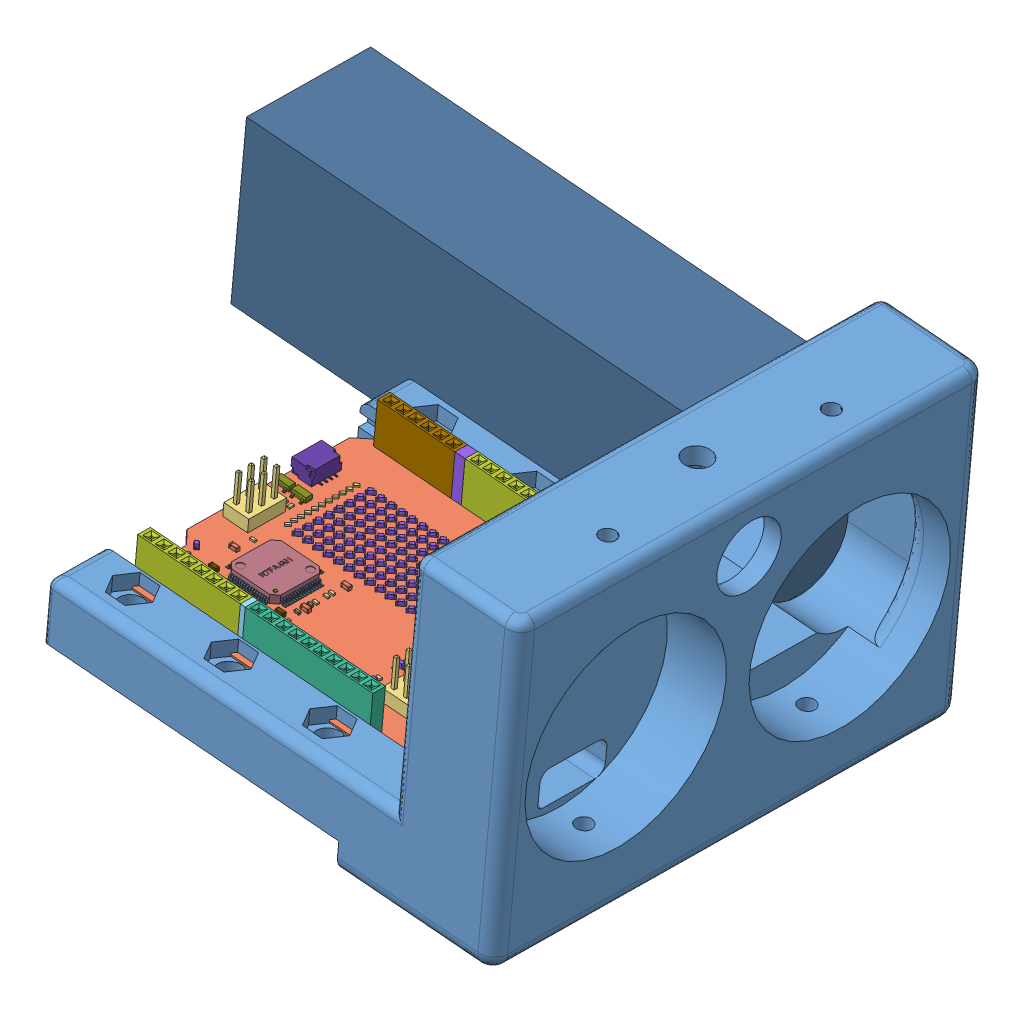
SolidWorks assembly SensorboxController1, configuration Standard. Lengths in mm. (continued)
Components (placement in the parent): (continued)
- PCB(ABX00087).step-1: PCB(ABX00087).step [Standard] at (42.9255 -81.7651 134.9822) x (-0.996616 0.082156 -0.002776) z (0.08218 0.996566 -0.010101) size (70.54 53.34 14.5) (continued)
  - U4.step-1: U4.step [Standard] at origin size (4 2 0.55) (continued)
    - IC_Texas_Instruments_TXB0108DQSR_eec.step-1: IC_Texas_Instruments_TXB0108DQSR_eec.step [Standard] at (13.565 34.6878 0.3) x (1 0 0) z (0 0 1) size (4 2 0.55) (continued)
      - Part16_MIR.step-2: Part16_MIR.step [Standard] at (3.331 -0.6643 -0.3) x (1 0 0) z (0 0 -1) size (0.2 0.55 0.1)
      - Part16_MIR1.step-1: Part16_MIR1.step [Standard] at (4.131 -0.6643 -0.3) x (1 0 0) z (0 0 -1) size (0.2 0.55 0.1)
      - Part16_MIR1.step-2: Part16_MIR1.step [Standard] at (4.531 -0.6643 -0.3) x (1 0 0) z (0 0 -1) size (0.2 0.55 0.1)
      - Part16_MIR1.step-3: Part16_MIR1.step [Standard] at (4.931 -0.6643 -0.3) x (1 0 0) z (0 0 -1) size (0.2 0.55 0.1)
      - Part16_MIR1.step-4: Part16_MIR1.step [Standard] at (5.331 -0.6643 -0.3) x (1 0 0) z (0 0 -1) size (0.2 0.55 0.1)
      - Part16_MIR1.step-5: Part16_MIR1.step [Standard] at (5.731 -0.6643 -0.3) x (1 0 0) z (0 0 -1) size (0.2 0.55 0.1)
      - Part16_MIR1.step-6: Part16_MIR1.step [Standard] at (6.131 -0.6643 -0.3) x (1 0 0) z (0 0 -1) size (0.2 0.55 0.1)
      - Part16_MIR1.step-7: Part16_MIR1.step [Standard] at (6.531 -0.6643 -0.3) x (1 0 0) z (0 0 -1) size (0.2 0.55 0.1)
      - Part16_MIR1.step-8: Part16_MIR1.step [Standard] at (6.931 -0.6643 -0.3) x (1 0 0) z (0 0 -1) size (0.2 0.55 0.1)
      - Part16 - Copy.step-1: Part16 - Copy.step [Standard] at (3.331 -2.0643 -0.3) size (0.2 0.65 0.1)
  - C24.step-1: C24.step [Standard] at origin size (0.5 1 0.5)
    - CAP-0402.step-1: CAP-0402.step [Standard] at (18.146 36.576 0) x (0 -1 0) z (0 0 1) size (1 0.5 0.5)
  - C25.step-1: C25.step [Standard] at origin size (0.5 1 0.5)
    - CAP-0402.step-1: CAP-0402.step [Standard] at (19.246 36.576 0) x (0 -1 0) z (0 0 1) size (1 0.5 0.5)
  - C26.step-1: C26.step [Standard] at origin size (0.5 1 0.5)
    - CAP-0402.step-1: CAP-0402.step [Standard] at (15.796 33.276 0) x (0 1 0) z (0 0 1) size (1 0.5 0.5)
  - U3.step-1: U3.step [Standard] at origin size (4 3 1)
    - 6430905744.step-1: 6430905744.step [Standard] at (26.825 22.1 0) x (0 1 0) z (0 0 1) size (3 4 1)
      - Body-3.step-1: Body-3.step [Standard] at (-1.5 -2 0) size (3 4 1)
        - Open CASCADE STEP translator 6.8 36.2.1.step-1: Open CASCADE STEP translator 6.8 36.2.1.step [Standard] at origin size (3 4 1)
      - Pin_Shape.step-1: Pin_Shape.step [Standard] at (-1.5 -1.3675 0) size (0.4 0.23 0.2)
        - Open CASCADE STEP translator 6.8 36.4.1.step-1: Open CASCADE STEP translator 6.8 36.4.1.step [Standard] at origin size (0.4 0.23 0.2)
      - Pin_Shape.step-2: Pin_Shape.step [Standard] at (1.5 1.3675 0) x (-1 0 0) z (0 0 1) size (0.4 0.23 0.2)
        - Open CASCADE STEP translator 6.8 36.4.1.step-1: Open CASCADE STEP translator 6.8 36.4.1.step [Standard] at origin size (0.4 0.23 0.2)
      - Pin_Shape.step-3: Pin_Shape.step [Standard] at (-1.5 -0.8675 0) size (0.4 0.23 0.2)
        - Open CASCADE STEP translator 6.8 36.4.1.step-1: Open CASCADE STEP translator 6.8 36.4.1.step [Standard] at origin size (0.4 0.23 0.2)
      - Pin_Shape.step-4: Pin_Shape.step [Standard] at (1.5 0.8675 0) x (-1 0 0) z (0 0 1) size (0.4 0.23 0.2)
        - Open CASCADE STEP translator 6.8 36.4.1.step-1: Open CASCADE STEP translator 6.8 36.4.1.step [Standard] at origin size (0.4 0.23 0.2)
      - Pin_Shape.step-5: Pin_Shape.step [Standard] at (-1.5 -0.3675 0) size (0.4 0.23 0.2)
        - Open CASCADE STEP translator 6.8 36.4.1.step-1: Open CASCADE STEP translator 6.8 36.4.1.step [Standard] at origin size (0.4 0.23 0.2)
      - Pin_Shape.step-6: Pin_Shape.step [Standard] at (1.5 0.3675 0) x (-1 0 0) z (0 0 1) size (0.4 0.23 0.2)
        - Open CASCADE STEP translator 6.8 36.4.1.step-1: Open CASCADE STEP translator 6.8 36.4.1.step [Standard] at origin size (0.4 0.23 0.2)
      - Pin_Shape.step-7: Pin_Shape.step [Standard] at (-1.5 0.1325 0) size (0.4 0.23 0.2)
        - Open CASCADE STEP translator 6.8 36.4.1.step-1: Open CASCADE STEP translator 6.8 36.4.1.step [Standard] at origin size (0.4 0.23 0.2)
      - Pin_Shape.step-8: Pin_Shape.step [Standard] at (1.5 -0.1325 0) x (-1 0 0) z (0 0 1) size (0.4 0.23 0.2)
        - Open CASCADE STEP translator 6.8 36.4.1.step-1: Open CASCADE STEP translator 6.8 36.4.1.step [Standard] at origin size (0.4 0.23 0.2)
      - Pin_Shape.step-9: Pin_Shape.step [Standard] at (-1.5 0.6325 0) size (0.4 0.23 0.2)
        - Open CASCADE STEP translator 6.8 36.4.1.step-1: Open CASCADE STEP translator 6.8 36.4.1.step [Standard] at origin size (0.4 0.23 0.2)
      - Pin_Shape.step-10: Pin_Shape.step [Standard] at (1.5 -0.6325 0) x (-1 0 0) z (0 0 1) size (0.4 0.23 0.2)
        - Open CASCADE STEP translator 6.8 36.4.1.step-1: Open CASCADE STEP translator 6.8 36.4.1.step [Standard] at origin size (0.4 0.23 0.2)
      - Pin_Shape.step-11: Pin_Shape.step [Standard] at (-1.5 1.1325 0) size (0.4 0.23 0.2)
        - Open CASCADE STEP translator 6.8 36.4.1.step-1: Open CASCADE STEP translator 6.8 36.4.1.step [Standard] at origin size (0.4 0.23 0.2)
      - Pin_Shape.step-12: Pin_Shape.step [Standard] at (1.5 -1.1325 0) x (-1 0 0) z (0 0 1) size (0.4 0.23 0.2)
        - Open CASCADE STEP translator 6.8 36.4.1.step-1: Open CASCADE STEP translator 6.8 36.4.1.step [Standard] at origin size (0.4 0.23 0.2)
      - Open CASCADE STEP translator 6.8 36.1.step-1: Open CASCADE STEP translator 6.8 36.1.step [Standard] at (-1.5 -2 0) size (0.38 0.38 0)
      - Thermal_Shape.step-1: Thermal_Shape.step [Standard] at (-0.8375 -1.6375 -0.001) size (1.68 3.28 0)
  - U1.step-1: U1.step [Standard] at origin size (12.2 12.2 1.68)
    - RA4M1 v4.step-1: RA4M1 v4.step [Standard] at (40.7498 25.853 0) size (12.2 12.2 1.67)
      - Designator1.step-1: Designator1.step [Standard] at origin size (12.2 12.2 1.67)
        - 6422462560.step-1: 6422462560.step [Standard] at (12 10 0) size (12.2 12.2 1.65)
          - Body-4.step-1: Body-4.step [Standard] at (-5 -5 0) size (10 10 1.65)
            - Open CASCADE STEP translator 6.8 23.1.1.step-1: Open CASCADE STEP translator 6.8 23.1.1.step [Standard] at origin size (10 10 1.65)
          - Leader-2.step-1: Leader-2.step [Standard] at (-5 -3.75 0) x (-1 0 0) z (0 0 1) size (1.1 0.27 0.88)
          - Leader-2.step-2: Leader-2.step [Standard] at (-3.75 5 0) x (0 1 0) z (0 0 1) size (1.1 0.27 0.88)
          - Leader-2.step-3: Leader-2.step [Standard] at (5 -3.75 0) size (1.1 0.27 0.88)
          - Leader-2.step-4: Leader-2.step [Standard] at (-3.75 -5 0) x (0 -1 0) z (0 0 1) size (1.1 0.27 0.88)
          - Leader-2.step-5: Leader-2.step [Standard] at (-5 -3.25 0) x (-1 0 0) z (0 0 1) size (1.1 0.27 0.88)
          - Leader-2.step-6: Leader-2.step [Standard] at (-3.25 5 0) x (0 1 0) z (0 0 1) size (1.1 0.27 0.88)
          - Leader-2.step-7: Leader-2.step [Standard] at (5 -3.25 0) size (1.1 0.27 0.88)
          - Leader-2.step-8: Leader-2.step [Standard] at (-3.25 -5 0) x (0 -1 0) z (0 0 1) size (1.1 0.27 0.88)
          - Leader-2.step-9: Leader-2.step [Standard] at (-5 -2.75 0) x (-1 0 0) z (0 0 1) size (1.1 0.27 0.88)
          - Leader-2.step-10: Leader-2.step [Standard] at (-2.75 5 0) x (0 1 0) z (0 0 1) size (1.1 0.27 0.88)
          - Leader-2.step-11: Leader-2.step [Standard] at (5 -2.75 0) size (1.1 0.27 0.88)
          - Leader-2.step-12: Leader-2.step [Standard] at (-2.75 -5 0) x (0 -1 0) z (0 0 1) size (1.1 0.27 0.88)
          - Leader-2.step-13: Leader-2.step [Standard] at (-5 -2.25 0) x (-1 0 0) z (0 0 1) size (1.1 0.27 0.88)
          - Leader-2.step-14: Leader-2.step [Standard] at (-2.25 5 0) x (0 1 0) z (0 0 1) size (1.1 0.27 0.88)
          - Leader-2.step-15: Leader-2.step [Standard] at (5 -2.25 0) size (1.1 0.27 0.88)
          - Leader-2.step-16: Leader-2.step [Standard] at (-2.25 -5 0) x (0 -1 0) z (0 0 1) size (1.1 0.27 0.88)
          - Leader-2.step-17: Leader-2.step [Standard] at (-5 -1.75 0) x (-1 0 0) z (0 0 1) size (1.1 0.27 0.88)
          - Leader-2.step-18: Leader-2.step [Standard] at (-1.75 5 0) x (0 1 0) z (0 0 1) size (1.1 0.27 0.88)
          - Leader-2.step-19: Leader-2.step [Standard] at (5 -1.75 0) size (1.1 0.27 0.88)
          - Leader-2.step-20: Leader-2.step [Standard] at (-1.75 -5 0) x (0 -1 0) z (0 0 1) size (1.1 0.27 0.88)
          - Leader-2.step-21: Leader-2.step [Standard] at (-5 -1.25 0) x (-1 0 0) z (0 0 1) size (1.1 0.27 0.88)
          - Leader-2.step-22: Leader-2.step [Standard] at (-1.25 5 0) x (0 1 0) z (0 0 1) size (1.1 0.27 0.88)
          - Leader-2.step-23: Leader-2.step [Standard] at (5 -1.25 0) size (1.1 0.27 0.88)
          - Leader-2.step-24: Leader-2.step [Standard] at (-1.25 -5 0) x (0 -1 0) z (0 0 1) size (1.1 0.27 0.88)
          - Leader-2.step-25: Leader-2.step [Standard] at (-5 -0.75 0) x (-1 0 0) z (0 0 1) size (1.1 0.27 0.88)
          - Leader-2.step-26: Leader-2.step [Standard] at (-0.75 5 0) x (0 1 0) z (0 0 1) size (1.1 0.27 0.88)
          - Leader-2.step-27: Leader-2.step [Standard] at (5 -0.75 0) size (1.1 0.27 0.88)
          - Leader-2.step-28: Leader-2.step [Standard] at (-0.75 -5 0) x (0 -1 0) z (0 0 1) size (1.1 0.27 0.88)
          - Leader-2.step-29: Leader-2.step [Standard] at (-5 -0.25 0) x (-1 0 0) z (0 0 1) size (1.1 0.27 0.88)
          - Leader-2.step-30: Leader-2.step [Standard] at (-0.25 5 0) x (0 1 0) z (0 0 1) size (1.1 0.27 0.88)
          - Leader-2.step-31: Leader-2.step [Standard] at (5 -0.25 0) size (1.1 0.27 0.88)
          - Leader-2.step-32: Leader-2.step [Standard] at (-0.25 -5 0) x (0 -1 0) z (0 0 1) size (1.1 0.27 0.88)
          - Leader-2.step-33: Leader-2.step [Standard] at (-5 0.25 0) x (-1 0 0) z (0 0 1) size (1.1 0.27 0.88)
          - Leader-2.step-34: Leader-2.step [Standard] at (0.25 5 0) x (0 1 0) z (0 0 1) size (1.1 0.27 0.88)
          - Leader-2.step-35: Leader-2.step [Standard] at (5 0.25 0) size (1.1 0.27 0.88)
          - Leader-2.step-36: Leader-2.step [Standard] at (0.25 -5 0) x (0 -1 0) z (0 0 1) size (1.1 0.27 0.88)
          - Leader-2.step-37: Leader-2.step [Standard] at (-5 0.75 0) x (-1 0 0) z (0 0 1) size (1.1 0.27 0.88)
          - Leader-2.step-38: Leader-2.step [Standard] at (0.75 5 0) x (0 1 0) z (0 0 1) size (1.1 0.27 0.88)
          - Leader-2.step-39: Leader-2.step [Standard] at (5 0.75 0) size (1.1 0.27 0.88)
          - Leader-2.step-40: Leader-2.step [Standard] at (0.75 -5 0) x (0 -1 0) z (0 0 1) size (1.1 0.27 0.88)
          - Leader-2.step-41: Leader-2.step [Standard] at (-5 1.25 0) x (-1 0 0) z (0 0 1) size (1.1 0.27 0.88)
          - Leader-2.step-42: Leader-2.step [Standard] at (1.25 5 0) x (0 1 0) z (0 0 1) size (1.1 0.27 0.88)
          - Leader-2.step-43: Leader-2.step [Standard] at (5 1.25 0) size (1.1 0.27 0.88)
          - Leader-2.step-44: Leader-2.step [Standard] at (1.25 -5 0) x (0 -1 0) z (0 0 1) size (1.1 0.27 0.88)
          - Leader-2.step-45: Leader-2.step [Standard] at (-5 1.75 0) x (-1 0 0) z (0 0 1) size (1.1 0.27 0.88)
          - Leader-2.step-46: Leader-2.step [Standard] at (1.75 5 0) x (0 1 0) z (0 0 1) size (1.1 0.27 0.88)
          - Leader-2.step-47: Leader-2.step [Standard] at (5 1.75 0) size (1.1 0.27 0.88)
          - Leader-2.step-48: Leader-2.step [Standard] at (1.75 -5 0) x (0 -1 0) z (0 0 1) size (1.1 0.27 0.88)
          - Leader-2.step-49: Leader-2.step [Standard] at (-5 2.25 0) x (-1 0 0) z (0 0 1) size (1.1 0.27 0.88)
          - Leader-2.step-50: Leader-2.step [Standard] at (2.25 5 0) x (0 1 0) z (0 0 1) size (1.1 0.27 0.88)
          - Leader-2.step-51: Leader-2.step [Standard] at (5 2.25 0) size (1.1 0.27 0.88)
          - Leader-2.step-52: Leader-2.step [Standard] at (2.25 -5 0) x (0 -1 0) z (0 0 1) size (1.1 0.27 0.88)
          - Leader-2.step-53: Leader-2.step [Standard] at (-5 2.75 0) x (-1 0 0) z (0 0 1) size (1.1 0.27 0.88)
          - Leader-2.step-54: Leader-2.step [Standard] at (2.75 5 0) x (0 1 0) z (0 0 1) size (1.1 0.27 0.88)
          - Leader-2.step-55: Leader-2.step [Standard] at (5 2.75 0) size (1.1 0.27 0.88)
          - Leader-2.step-56: Leader-2.step [Standard] at (2.75 -5 0) x (0 -1 0) z (0 0 1) size (1.1 0.27 0.88)
          - Leader-2.step-57: Leader-2.step [Standard] at (-5 3.25 0) x (-1 0 0) z (0 0 1) size (1.1 0.27 0.88)
          - Leader-2.step-58: Leader-2.step [Standard] at (3.25 5 0) x (0 1 0) z (0 0 1) size (1.1 0.27 0.88)
          - Leader-2.step-59: Leader-2.step [Standard] at (5 3.25 0) size (1.1 0.27 0.88)
          - Leader-2.step-60: Leader-2.step [Standard] at (3.25 -5 0) x (0 -1 0) z (0 0 1) size (1.1 0.27 0.88)
          - Leader-2.step-61: Leader-2.step [Standard] at (-5 3.75 0) x (-1 0 0) z (0 0 1) size (1.1 0.27 0.88)
          - Leader-2.step-62: Leader-2.step [Standard] at (3.75 5 0) x (0 1 0) z (0 0 1) size (1.1 0.27 0.88)
          - Leader-2.step-63: Leader-2.step [Standard] at (5 3.75 0) size (1.1 0.27 0.88)
          - Leader-2.step-64: Leader-2.step [Standard] at (3.75 -5 0) x (0 -1 0) z (0 0 1) size (1.1 0.27 0.88)
        - 7219473552.step-1: 7219473552.step [Standard] at (8.2001 13.7999 0.25) size (0.7 0.7 1.42)
          - Extruded-3.step-1: Extruded-3.step [Standard] at origin size (0.7 0.7 1.42)
    - 6360838992.step-1: 6360838992.step [Standard] at (48.9498 39.6529 0.25) size (0.7 0.71 1.43)
      - Extruded-4.step-1: Extruded-4.step [Standard] at origin size (0.7 0.71 1.43)
  - R23.step-1: R23.step [Standard] at origin size (1 0.5 0.34)
    - RES-0402.step-1: RES-0402.step [Standard] at (26.416 35.433 0) size (1 0.5 0.34)
  - R40.step-1: R40.step [Standard] at origin size (0.5 1 0.34)
    - RES-0402.step-1: RES-0402.step [Standard] at (25.125 25.3 0) x (0 -1 0) z (0 0 1) size (1 0.5 0.34)
  - R38.step-1: R38.step [Standard] at origin size (0.5 1 0.34)
    - RES-0402.step-1: RES-0402.step [Standard] at (26.225 25.3 0) x (0 -1 0) z (0 0 1) size (1 0.5 0.34)
  - R36.step-1: R36.step [Standard] at origin size (1 0.5 0.34)
    - RES-0402.step-1: RES-0402.step [Standard] at (27.95 27.235 0) x (-1 0 0) z (0 0 1) size (1 0.5 0.34)
  - R44.step-1: R44.step [Standard] at origin size (0.5 1 0.34)
    - RES-0402.step-1: RES-0402.step [Standard] at (22.925 23 0) x (0 1 0) z (0 0 1) size (1 0.5 0.34)
  - R43.step-1: R43.step [Standard] at origin size (0.5 1 0.34)
    - RES-0402.step-1: RES-0402.step [Standard] at (22.925 25.3 0) x (0 -1 0) z (0 0 1) size (1 0.5 0.34)
  - R7.step-1: R7.step [Standard] at origin size (1 0.5 0.34)
    - RES-0402.step-1: RES-0402.step [Standard] at (60.646 32.376 0) x (-1 0 0) z (0 0 1) size (1 0.5 0.34)
  - R1.step-1: R1.step [Standard] at origin size (0.5 1 0.34)
    - RES-0402.step-1: RES-0402.step [Standard] at (13.125 34.231 0) x (0 1 0) z (0 0 1) size (1 0.5 0.34)
  - L3.step-1: L3.step [Standard] at origin size (4.8 4.8 2)
    - 6431045296.step-1: 6431045296.step [Standard] at (29.5083 17.2482 0.05) size (4.8 4.8 2)
      - Extruded-5.step-1: Extruded-5.step [Standard] at origin size (4.8 4.8 2)
  - L2.step-1: L2.step [Standard] at origin size (1.6 0.8 0.8)
    - FER-0603.step-1: FER-0603.step [Standard] at (59.5098 41.428 0) x (1 0 0) z (0 0 1) size (1.6 0.8 0.8)
  - L1.step-1: L1.step [Standard] at origin size (1.6 0.8 0.8)
    - FER-0603.step-1: FER-0603.step [Standard] at (45.9897 41.428 0) x (1 0 0) z (0 0 1) size (1.6 0.8 0.8)
  - C16.step-1: C16.step [Standard] at origin size (2 1.25 1.25)
    - CAP-0805.step-1: CAP-0805.step [Standard] at (30.6599 23.2481 0) x (-1 0 0) z (0 0 1) size (2 1.25 1.25)
  - C11.step-1: C11.step [Standard] at origin size (0.5 1 0.5)
    - CAP-0402.step-1: CAP-0402.step [Standard] at (19.19 9.991 0) x (0 1 0) z (0 0 1) size (1 0.5 0.5)
  - C19.step-1: C19.step [Standard] at origin size (1.25 2 1.25)
    - CAP-0805.step-1: CAP-0805.step [Standard] at (25.2157 17.2529 0) x (0 -1 0) z (0 0 1) size (2 1.25 1.25)
  - C14.step-1: C14.step [Standard] at origin size (0.5 1 0.5)
    - CAP-0402.step-1: CAP-0402.step [Standard] at (27.325 25.3 0) x (0 1 0) z (0 0 1) size (1 0.5 0.5)
  - C15.step-1: C15.step [Standard] at origin size (2 1.25 1.25)
    - CAP-0805.step-1: CAP-0805.step [Standard] at (30.6599 21.2981 0) x (-1 0 0) z (0 0 1) size (2 1.25 1.25)
  - C13.step-1: C13.step [Standard] at origin size (1.25 2 1.25)
    - CAP-0805.step-1: CAP-0805.step [Standard] at (23.199 17.2531 0) x (0 1 0) z (0 0 1) size (2 1.25 1.25)
  - C12.step-1: C12.step [Standard] at origin size (1 0.5 0.5)
    - CAP-0402.step-1: CAP-0402.step [Standard] at (25.6 19.6 0) size (1 0.5 0.5)
  - C20.step-1: C20.step [Standard] at origin size (0.5 1 0.5)
    - CAP-0402.step-1: CAP-0402.step [Standard] at (28.425 25.3 0) x (0 1 0) z (0 0 1) size (1 0.5 0.5)
  - C9.step-1: C9.step [Standard] at origin size (1.6 0.8 0.8)
    - CAP-0603.step-1: CAP-0603.step [Standard] at (44.3498 37.953 0) size (1.6 0.8 0.8)
  - C8.step-1: C8.step [Standard] at origin size (1 0.5 0.5)
    - CAP-0402.step-1: CAP-0402.step [Standard] at (44.6495 39.306 0) size (1 0.5 0.5)
  - C6.step-1: C6.step [Standard] at origin size (1 0.5 0.5)
    - CAP-0402.step-1: CAP-0402.step [Standard] at (59.2348 42.628 0) size (1 0.5 0.5)
  - C3.step-1: C3.step [Standard] at origin size (1 0.5 0.5)
    - CAP-0402.step-1: CAP-0402.step [Standard] at (44.646 36.776 0) size (1 0.5 0.5)
  - C2.step-1: C2.step [Standard] at origin size (1.6 0.8 0.8)
    - CAP-0603.step-1: CAP-0603.step [Standard] at (60.946 35.876 0) x (-1 0 0) z (0 0 1) size (1.6 0.8 0.8)
  - R51.step-1: R51.step [Standard] at origin size (1 0.5 0.34)
    - RES-0402.step-1: RES-0402.step [Standard] at (9.125 41.6599 0) x (-1 0 0) z (0 0 1) size (1 0.5 0.34)
  - R50.step-1: R50.step [Standard] at origin size (1 0.5 0.34)
    - RES-0402.step-1: RES-0402.step [Standard] at (9.125 40.466 0) x (-1 0 0) z (0 0 1) size (1 0.5 0.34)
  - R15.step-1: R15.step [Standard] at origin size (1 0.5 0.34)
    - RES-0402.step-1: RES-0402.step [Standard] at (44.646 33.476 0) size (1 0.5 0.34)
  - R18.step-1: R18.step [Standard] at origin size (0.5 1 0.34)
    - RES-0402.step-1: RES-0402.step [Standard] at (11.925 31.466 0) x (0 -1 0) z (0 0 1) size (1 0.5 0.34)
  - R24.step-1: R24.step [Standard] at origin size (0.5 1 0.34)
    - RES-0402.step-1: RES-0402.step [Standard] at (64.3844 41.9405 0) x (0 -1 0) z (0 0 1) size (1 0.5 0.34)
  - R19.step-1: R19.step [Standard] at origin size (1 0.5 0.34)
    - RES-0402.step-1: RES-0402.step [Standard] at (44.646 32.376 0) size (1 0.5 0.34)
  - R49.step-1: R49.step [Standard] at origin size (0.5 1 0.34)
    - RES-0402.step-1: RES-0402.step [Standard] at (21.596 33.276 0) x (0 1 0) z (0 0 1) size (1 0.5 0.34)
  - R25.step-1: R25.step [Standard] at origin size (1 0.5 0.34)
    - RES-0402.step-1: RES-0402.step [Standard] at (26.416 43.307 0) size (1 0.5 0.34)
  - DL3.step-1: DL3.step [Standard] at origin size (1.7 1.7 0.8)
    - HSMx-190.step-1: HSMx-190.step [Standard] at (64.897 39.5529 0) x (0.707107 -0.707107 0) z (0 0 1) size (1.6 0.8 0.8)
  - C21.step-1: C21.step [Standard] at origin size (2 1.25 1.25)
    - CAP-0805.step-1: CAP-0805.step [Standard] at (1.8498 44.1531 0) size (2 1.25 1.25)
  - R22.step-1: R22.step [Standard] at origin size (1 0.5 0.34)
    - RES-0402.step-1: RES-0402.step [Standard] at (26.416 37.719 0) size (1 0.5 0.34)
  - DL2.step-1: DL2.step [Standard] at origin size (1.6 0.8 0.8)
    - HSMx-190.step-1: HSMx-190.step [Standard] at (26.416 34.29 0) x (1 0 0) z (0 0 1) size (1.6 0.8 0.8)
  - DL1.step-1: DL1.step [Standard] at origin size (1.6 0.8 0.8)
    - HSMx-190.step-1: HSMx-190.step [Standard] at (26.416 36.576 0) x (1 0 0) z (0 0 1) size (1.6 0.8 0.8)
  - DL4.step-1: DL4.step [Standard] at origin size (1.6 0.8 0.8)
    - HSMx-190.step-1: HSMx-190.step [Standard] at (26.416 42.164 0) x (1 0 0) z (0 0 1) size (1.6 0.8 0.8)
  - R17.step-1: R17.step [Standard] at origin size (0.5 1 0.34)
    - RES-0402.step-1: RES-0402.step [Standard] at (13.125 31.4599 0) x (0 -1 0) z (0 0 1) size (1 0.5 0.34)
  - C7.step-1: C7.step [Standard] at origin size (1 0.5 0.5)
    - CAP-0402.step-1: CAP-0402.step [Standard] at (46.2648 42.628 0) size (1 0.5 0.5)
  - J5.step-1: J5.step [Standard] at origin size (14.4 9.4 14.5)
    - pj-102ah.step-1: pj-102ah.step [Standard] at (-1.96 8.3559 5.3937) x (-1 0 0) z (0 1 0) size (14.4 14.5 9.4)
  - D2.step-1: D2.step [Standard] at origin size (2.01 3.7 1.2)
    - SOD123FL.step-1: SOD123FL.step [Standard] at (28.396 26.476 0) x (0 1 0) z (0 0 1) size (3.7 2 1.2)
      - 8279795424.step-1: 8279795424.step [Standard] at (4 2 0) size (3.7 2 1.2)
        - Body-2.step-1: Body-2.step [Standard] at (-1.5 -1 0) size (3 2 1.2)
          - Open CASCADE STEP translator 7.5 15.1.1.step-1: Open CASCADE STEP translator 7.5 15.1.1.step [Standard] at origin size (3 2 1.2)
        - Lead.step-1: Lead.step [Standard] at (-1.85 -0.425 0) size (1.65 0.75 1.01)
        - Lead.step-2: Lead.step [Standard] at (1.85 0.425 0) x (-1 0 0) z (0 0 1) size (1.65 0.75 1.01)
  - D3.step-1: D3.step [Standard] at origin size (2.9 2.31 1)
    - PRTR5V0U2X.step-1: PRTR5V0U2X.step [Standard] at (9.125 37.866 0) x (-1 0 0) z (0 0 1) size (2.9 2.31 1)
  - J3.step-1: J3.step [Standard] at origin size (5.04 7.62 11.5)
    - 2x3 Header.step-1: 2x3 Header.step [Standard] at (67.4371 24.1301 0) x (-1 0 0) z (0 1 0) size (5.04 11.5 7.62)
  - PB1.step-1: PB1.step [Standard] at origin size (8.2 6.5 2.66)
    - TETactileSwitch1571636.step-1: TETactileSwitch1571636.step [Standard] at (6.3501 49.4031 2) size (8.2 6.5 2.66)
  - R39.step-1: R39.step [Standard] at origin size (1 0.5 0.34)
    - RES-0402.step-1: RES-0402.step [Standard] at (4.5498 43.853 0) x (-1 0 0) z (0 0 1) size (1 0.5 0.34)
  - J1.step-1: J1.step [Standard] at origin size (6.8 9.54 3.62)
    - CX90B-16P_CL0480-0755-0-00_3DDrawing_STEP_CX90B-16P_3D_48007525000_3D_STP.step-1: CX90B-16P_CL0480-0755-0-00_3DDrawing_STEP_CX90B-16P_3D_48007525000_3D_STP.step [Standard] at (3.8875 37.866 0.31) x (0 -1 0) z (0 0 1) size (9.54 6.8 3.62)
      - CX90B-16P_3D.step-1: CX90B-16P_3D.step [Standard] at (0.25 -4.65 1.28) x (1 0 0) z (0 -1 0) size (9.54 3.62 6.8)
  - JDIGITAL.step-1: JDIGITAL.step [Standard] at origin size (47.7 2.54 11.7)
    - 6431046176.step-1: 6431046176.step [Standard] at (43.6689 50.7997 0) size (0.99 2.54 8.5)
      - Extruded-6.step-1: Extruded-6.step [Standard] at origin size (0.99 2.54 8.5)
    - Header_Fem_1X10_digikey.step-1: Header_Fem_1X10_digikey.step [Standard] at (30.226 50.8 0) x (-1 0 0) z (0 1 0) size (25.9 11.7 2.54)
    - Header _Fem_1X8.step-1: Header _Fem_1X8.step [Standard] at (54.57 50.8 0) x (-1 0 0) z (0 1 0) size (20.82 11.7 2.54)
  - JANALOG.step-1: JANALOG.step [Standard] at origin size (38.6 2.54 11.7)
    - 6431040416.step-1: 6431040416.step [Standard] at (48.2497 2.5405 0) size (2.04 2.54 8.5)
      - Extruded-7.step-1: Extruded-7.step [Standard] at origin size (2.04 2.54 8.5)
    - Header _Fem_1X8.step-1: Header _Fem_1X8.step [Standard] at (36.82 2.54 0) x (1 0 0) z (0 -1 0) size (20.82 11.7 2.54)
    - Header_Fem_1X6_digikey.step-1: Header_Fem_1X6_digikey.step [Standard] at (57.14 2.54 0) x (1 0 0) z (0 -1 0) size (15.74 11.7 2.54)
- battery3300a-1: battery3300a [Standard] at (-61.4562 -77.0758 102.7275) x (0.996616 -0.082156 0.002776) z (-0.001937 0.010295 0.999945) size (100 34 25)
Mates (geometry in assembly coordinates):
- Parallel1: parallel: plane of Sensorbox_small_arduino-1 through (42.5964 -79.6711 134.9776) normal (-0.08218 -0.996566 0.010101); line of PCB(ABX00087).step-1/Board.step-1/Open CASCADE STEP translator 7.5 4.1.1.step-1 through (41.8256 -81.1338 188.3165) axis (-0.996616 0.082156 -0.002776)
- Parallel2: parallel anti-aligned: plane of Sensorbox_small_arduino-1 through (42.3534 -83.7989 280.1467) normal (0.08218 0.996566 -0.010101); plane of PCB(ABX00087).step-1/Board.step-1/Open CASCADE STEP translator 7.5 4.1.1.step-1 through (9.221 -80.329 161.4762) normal (-0.08218 -0.996566 0.010101)
- Deckungsgleich3: coincident anti-aligned: plane of Sensorbox_small_arduino-1 through (44.4865 -57.9317 279.8845) normal (-0.996616 0.082156 -0.002776); plane of PCB(ABX00087).step-1/Board.step-1/Open CASCADE STEP translator 7.5 4.1.1.step-1 through (42.7915 -83.3556 135.9984) normal (0.996616 -0.082156 0.002776)
- Parallel4: parallel aligned: line of Sensorbox_small_arduino-1 through (11.7028 -74.8096 125.6672) axis (0.996616 -0.082156 0.002776); line of battery3300a-1 through (-61.5047 -76.8184 127.7262) axis (0.996616 -0.082156 0.002776)
